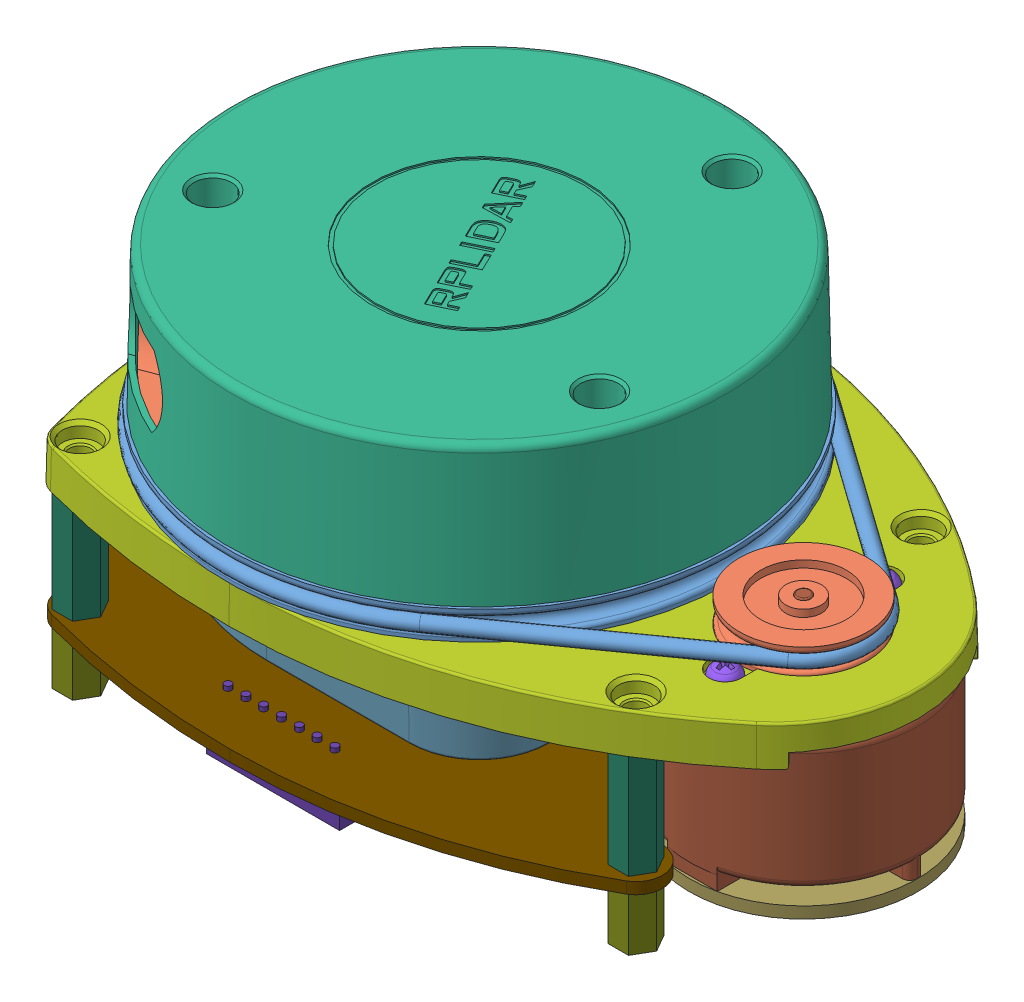
SolidWorks assembly RP-lidar-A1, configuration Default. Lengths in mm.
Overall size (114.01 53.5 94.54).
31 component instances, 20 part files, 0 mates.
Components (placement in the parent):
- RP-lidar-A1.iam-1: RP-lidar-A1.iam [Default] at origin size (114.01 53.5 94.54)
  - head-base.ipt-1: head-base.ipt [Default] at (-90.5533 751.2923 132.9176) x (0.900173 0 -0.435532) z (0.435532 0 0.900173) size (70.78 21.4 70.78)
  - detector-mount.ipt-1: detector-mount.ipt [Default] at (-90.4238 754.2923 132.7756) x (-0.437519 0 -0.899209) z (0.899209 0 -0.437519) size (22.83 18.52 24.93)
  - detector.ipt-1: detector.ipt [Default] at (-93.3269 763.2923 153.0936) x (-0.088661 0.979252 -0.182219) z (-0.899209 0 0.437519) size (14 14 11.5)
  - laser.ipt-1: laser.ipt [Default] at (-96.1268 764.2923 107.8262) x (0.382786 0.720375 0.578389) z (-0.833913 0 0.551896) size (6.5 6.5 21.2)
  - laser-mount.ipt-1: laser-mount.ipt [Default] at (-90.5533 755.2923 132.9176) x (-0.430466 0 -0.902607) z (0.902607 0 -0.430466) size (15.7 18.5 21.49)
  - head.ipt-1: head.ipt [Default] at (-90.5533 773.1923 132.9176) x (0.435532 0 0.900173) z (0.900173 0 -0.435532) size (70 19.5 70)
  - base.ipt-1: base.ipt [Default] at (-90.5533 748.2923 132.9176) size (96.74 12.7 70.28)
  - Woodscrews_GB_TYPE136 M2X6-N.ipt-1: Woodscrews_GB_TYPE136 M2X6-N.ipt [Default] at (-64.2029 766.7923 142.3864) x (0 -1 0) z (-0.876166 0 -0.482009) size (7.56 3.9 3.9)
  - Woodscrews_GB_TYPE136 M2X6-N.ipt-2: Woodscrews_GB_TYPE136 M2X6-N.ipt [Default] at (-81.6242 766.7923 106.3795) x (0 -1 0) z (-0.876166 0 -0.482009) size (7.56 3.9 3.9)
  - Woodscrews_GB_TYPE136 M2X6-N.ipt-3: Woodscrews_GB_TYPE136 M2X6-N.ipt [Default] at (-115.7581 766.7923 145.1125) x (0 -1 0) z (-0.922446 0 -0.386125) size (7.56 3.9 3.9)
  - Woodscrews_GB_TYPE136 M2X6-N.ipt-4: Woodscrews_GB_TYPE136 M2X6-N.ipt [Default] at (-45.0533 750.5923 121.9176) x (0 -1 0) z (0.032922 0 0.999458) size (7.56 3.9 3.9)
  - Woodscrews_GB_TYPE136 M2X6-N.ipt-5: Woodscrews_GB_TYPE136 M2X6-N.ipt [Default] at (-45.0533 750.5923 143.9176) x (0 -1 0) z (0.032922 0 0.999458) size (7.56 3.9 3.9)
  - motherboard.ipt-1: motherboard.ipt [Default] at (-90.5533 738.2923 132.9176) size (55.5 1 57)
  - connector-1_25-3pin.ipt-1: connector-1_25-3pin.ipt [Default] at (-57.5533 723.4923 132.5551) x (0 0 1) z (0 -1 0) size (8.9 5.2 3.4)
  - motor.ipt-1: motor.ipt [Default] at (-45.0533 728.7923 132.9176) x (0 0 1) z (-1 0 0) size (32 30.2 32)
  - motor-board.ipt-1: motor-board.ipt [Default] at (-45.0533 725.1923 132.9176) x (0.420142 0 0.907458) z (-0.907458 0 0.420142) size (32 1.6 32)
  - connector-1_25-4pin.ipt-1: connector-1_25-4pin.ipt [Default] at (-68.3533 736.4423 132.7926) x (0 0 1) z (1 0 0) size (10.15 4.2 4.7)
  - bottom-lid.ipt-1: bottom-lid.ipt [Default] at (-90.5533 737.2923 132.9176) size (60.06 11.01 60.34)
  - stand_15x2.ipt-1: stand_15x2.ipt [Default] at (-118.5533 729.2923 160.9176) size (5.77 15 5)
  - stand_15x2.ipt-2: stand_15x2.ipt [Default] at (-48.5533 729.2923 152.9176) size (5.77 15 5)
  - stand_15x2.ipt-3: stand_15x2.ipt [Default] at (-48.5533 729.2923 112.9176) size (5.77 15 5)
  - stand_15x2.ipt-4: stand_15x2.ipt [Default] at (-118.5533 729.2923 104.9176) size (5.77 15 5)
  - stand-8x2.ipt-1: stand-8x2.ipt [Default] at (-48.5533 727.6923 152.9176) x (1 0 0) z (0 0 -1) size (5.77 8 5)
  - stand-8x2.ipt-2: stand-8x2.ipt [Default] at (-118.5533 727.6923 160.9176) x (1 0 0) z (0 0 -1) size (5.77 8 5)
  - stand-8x2.ipt-3: stand-8x2.ipt [Default] at (-118.5533 727.6923 104.9176) x (1 0 0) z (0 0 -1) size (5.77 8 5)
  - stand-8x2.ipt-4: stand-8x2.ipt [Default] at (-48.5533 727.6923 112.9176) x (1 0 0) z (0 0 -1) size (5.77 8 5)
  - connector-7pin-2_5.ipt-1: connector-7pin-2_5.ipt [Default] at (-90.5533 727.6923 160.0176) x (0 -1 0) z (1 0 0) size (8.2 5 20)
  - devboard.ipt-1: devboard.ipt [Default] at (-90.5533 729.2923 132.9176) x (1 0 0) z (0 0 -1) size (80.7 7.64 70)
  - rubber.ipt-1: rubber.ipt [Default] at (-90.5533 751.4783 132.9176) x (1 0 0) z (0 -1 0) size (90.89 71.78 2)
  - wheel.ipt-1: wheel.ipt [Default] at (-45.0533 749.2923 132.9176) x (-0.124101 0 -0.99227) z (0.99227 0 -0.124101) size (18 5.5 18)
